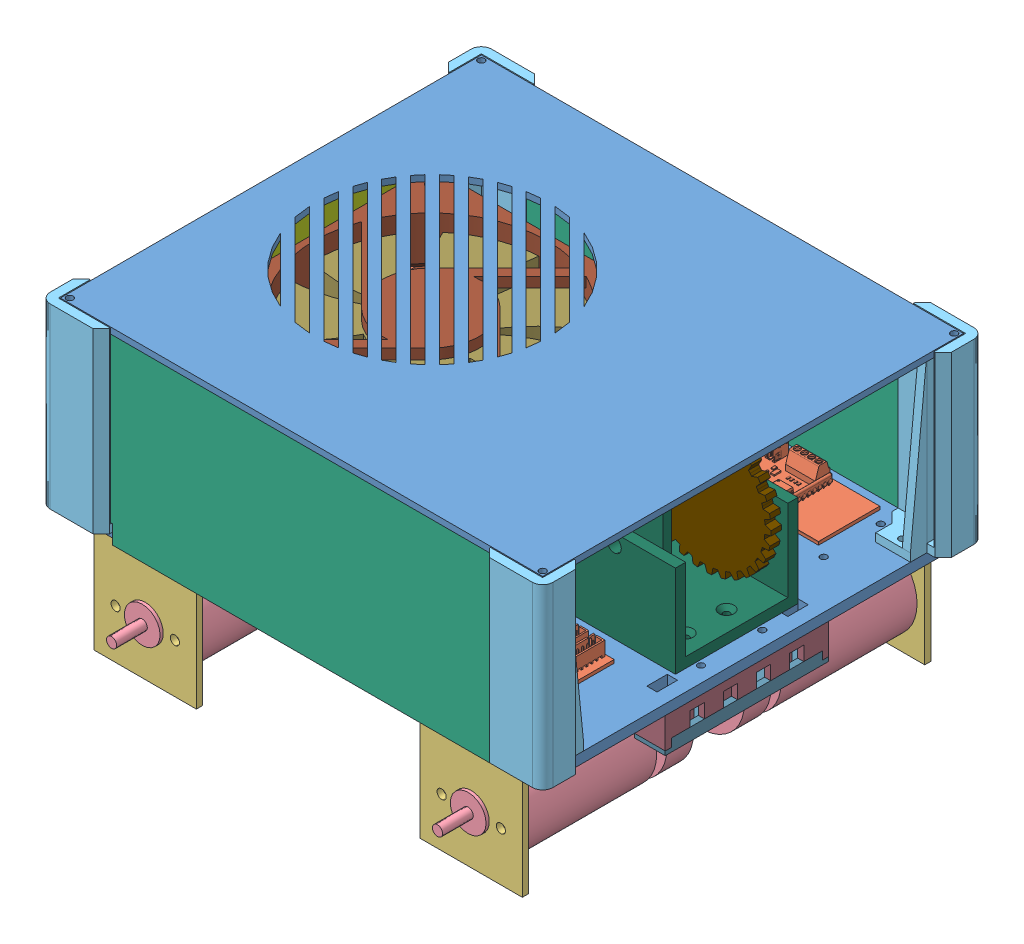
SolidWorks assembly SUM, configuration Standard. Lengths in mm.
Overall size (246 144 233).
34 component instances, 20 part files, 62 mates.
Components (placement in the parent):
- Part2^SUM-1: Part2^SUM [Standard] at origin (virtual)
- base_plate-1: base_plate [Standard] at (-44.1606 132.4921 37.7071) size (230 5 200)
- PCB_Chassisv1.0.step-1: PCB_Chassisv1.0.step [Standard] at (-139.1606 153.7785 -50.9871) x (0 0 1) z (0 1 0) size (160.04 200 38.68)
- motorhalter-1: motorhalter [Standard] at (40.8983 106.4921 129.0129) x (1 0 0) z (0 0 -1) size (50 52 55)
- motorhalter-2: motorhalter [Standard] at (-118.6423 106.4921 129.0129) x (1 0 0) z (0 0 -1) size (50 52 55)
- motorhalter-5: motorhalter [Standard] at (-119.1606 106.4921 -70.9871) x (-1 0 0) z (0 0 1) size (50 52 55)
- motorhalter-6: motorhalter [Standard] at (40.8394 106.4921 -70.9871) x (-1 0 0) z (0 0 1) size (50 52 55)
- motor-1: motor [Standard] at (-118.6423 104.4921 59.5129) size (42.5 42.5 104)
- motor-2: motor [Standard] at (40.8983 104.4921 59.5129) size (42.5 42.5 104)
- motor-3: motor [Standard] at (-119.1606 104.4921 -1.4871) x (1 0 0) z (0 0 -1) size (42.5 42.5 104)
- motor-4: motor [Standard] at (40.8394 104.4921 -1.4871) x (-1 0 0) z (0 0 -1) size (42.5 42.5 104)
- base-ecke-halter-2: base-ecke-halter [teil rechts] at (-147.1606 137.4921 -68.9871) x (0 0 -1) z (1 0 0) size (28 87 30)
- base-ecke-halter-3: base-ecke-halter [teil rechts] at (68.8394 137.4921 127.0129) x (0 0 1) z (-1 0 0) size (28 87 30)
- base-ecke-halter-6: base-ecke-halter [teil links] at (-147.1606 137.4921 127.0129) x (0 0 -1) z (1 0 0) size (28 87 30)
- base-ecke-halter-7: base-ecke-halter [teil links] at (68.8394 137.4921 -68.9871) x (0 0 1) z (-1 0 0) size (28 87 30)
- wall_L_R-1: wall_L_R [Standard] at (-39.1606 176.9921 129.0129) x (1 0 0) z (0 -1 0) size (227 3 89)
- wall_L_R-2: wall_L_R [Standard] at (-39.1606 176.9921 -73.9871) x (1 0 0) z (0 -1 0) size (227 3 89)
- wall_B-1: wall_B [Standard] at (-157.1606 176.9921 29.0129) x (0 0 -1) z (1 0 0) size (197 89 3)
- Funk.step-1: Funk.step [Standard] at (-80.8303 237.3371 119.9389) x (1 0 0) z (0 0 -1) size (61.6 64.9 16.02)
- LORA_mount-1: LORA_mount [Standard] at (-24.6323 144.9921 125.3504) x (-1 0 0) z (0 0 -1) size (70 75 15)
- Vent_mount-1: Vent_mount [Standard] at (-64.1606 178.4895 29.0129) x (0 0 1) z (-1 0 0) size (160 4 150)
- Vent.stp-1: Vent.stp [Standard] at (-139.9204 182.4895 90.0129) size (122.01 25.4 122.01)
  - FRAME.stp-1: FRAME.stp [Standard] at (61 0 -61) size (122.01 25.4 122.01)
  - 410005100005.stp-1: 410005100005.stp [Standard] at (61 2.0938 -61) x (1 0 0) z (0 -1 0) size (111.8 111.72 16)
- Scheinwerfer_Gehäuse-1: Scheinwerfer_Gehäuse [Standard] at (68.3394 132.4921 29.0129) x (0 0 1) z (1 0 0) size (80 15 15)
- Scheinwerfer_deckel-1: Scheinwerfer_deckel [Standard] at (68.3394 115.4921 29.0129) x (0 0 -1) z (1 0 0) size (80 6 15)
- Scheinwerfer_Gehäuse-2: Scheinwerfer_Gehäuse [Standard] at (-146.5449 132.4921 29.0134) x (0.007714 0 -0.99997) z (-0.99997 0 -0.007714) size (80 15 15)
- Scheinwerfer_deckel-2: Scheinwerfer_deckel [Standard] at (-146.5449 115.4921 29.0134) x (-0.007714 0 0.99997) z (-0.99997 0 -0.007714) size (80 6 15)
- seilwinde-1: seilwinde [Standard] at (70.9432 149.6596 27.3308) size (106.6 93.21 60)
  - seilwinde_case-1: seilwinde_case [Standard] at (-50.1038 -12.1675 -3.3179) size (90 45 60)
  - 858 Stepper Motor 5VDC.step-1: 858 Stepper Motor 5VDC.step [Standard] at (-72.6038 19.8325 -12.3221) x (-1 0 0) z (0 0 -1) size (42 34.5 29)
  - seilwinde_small_gear-1: seilwinde_small_gear [Standard] at (-72.5744 27.8557 -21.3221) x (1 0 0) z (0 -1 0) size (20.09 5 19.59)
  - seilwinde_big_gear-1: seilwinde_big_gear [Standard] at (-35.1038 27.8325 -17.1569) x (0.729284 -0.684211 0) z (0.684211 0.729284 0) size (65.88 15 66)
- roof1-1: roof1 [Standard] at (-39.1606 221.4921 29.0129) x (0 0 -1) z (1 0 0) size (206 3 236)
Mates (geometry in assembly coordinates):
- Slot1: slot anti-aligned: plane of motorhalter-1 through (49.6483 132.4921 115.7629) normal (0 0 1); cylinder of base_plate-1 through (52.3394 132.4921 118.0129) axis (0 1 0) radius 1.65; cylinder of motorhalter-1 through (55.1483 132.4921 118.0129) axis (0 -1 0) radius 2.25
- Slot2: slot anti-aligned: plane of motorhalter-1 through (26.6483 132.4921 115.7629) normal (0 0 1); cylinder of base_plate-1 through (29.3394 132.4921 118.0129) axis (0 1 0) radius 1.65; cylinder of motorhalter-1 through (32.1483 132.4921 118.0129) axis (0 -1 0) radius 2.25
- Coincident2: coincident anti-aligned: plane of base_plate-1 through (-44.1606 132.4921 37.7071) normal (0 -1 0); plane of motorhalter-1 through (15.8983 132.4921 126.0129) normal (0 1 0)
- Slot3: slot anti-aligned: plane of motorhalter-2 through (-132.8923 132.4921 115.7629) normal (0 0 1); cylinder of base_plate-1 through (-130.6606 132.4921 118.0129) axis (0 1 0) radius 1.65; cylinder of motorhalter-2 through (-127.3923 132.4921 118.0129) axis (0 -1 0) radius 2.25
- Slot4: slot anti-aligned: plane of motorhalter-2 through (-109.8923 132.4921 115.7629) normal (0 0 1); cylinder of base_plate-1 through (-107.6606 132.4921 118.0129) axis (0 1 0) radius 1.65; cylinder of motorhalter-2 through (-104.3923 132.4921 118.0129) axis (0 -1 0) radius 2.25
- Coincident3: coincident anti-aligned: plane of base_plate-1 through (-44.1606 132.4921 37.7071) normal (0 -1 0); plane of motorhalter-2 through (-143.6423 132.4921 126.0129) normal (0 1 0)
- Slot5: slot anti-aligned: plane of motorhalter-5 through (-127.9106 132.4921 -57.7371) normal (0 0 -1); cylinder of base_plate-1 through (-130.6606 132.4921 -59.9871) axis (0 1 0) radius 1.65; cylinder of motorhalter-5 through (-133.4106 132.4921 -59.9871) axis (0 -1 0) radius 2.25
- Slot6: slot anti-aligned: plane of motorhalter-5 through (-104.9106 132.4921 -57.7371) normal (0 0 -1); cylinder of base_plate-1 through (-107.6606 132.4921 -59.9871) axis (0 1 0) radius 1.65; cylinder of motorhalter-5 through (-110.4106 132.4921 -59.9871) axis (0 -1 0) radius 2.25
- Slot7: slot anti-aligned: plane of motorhalter-6 through (32.0894 132.4921 -57.7371) normal (0 0 -1); cylinder of base_plate-1 through (29.3394 132.4921 -59.9871) axis (0 1 0) radius 1.65; cylinder of motorhalter-6 through (26.5894 132.4921 -59.9871) axis (0 -1 0) radius 2.25
- Slot8: slot anti-aligned: plane of motorhalter-6 through (55.0894 132.4921 -57.7371) normal (0 0 -1); cylinder of base_plate-1 through (52.3394 132.4921 -59.9871) axis (0 1 0) radius 1.65; cylinder of motorhalter-6 through (49.5894 132.4921 -59.9871) axis (0 -1 0) radius 2.25
- Coincident4: coincident anti-aligned: plane of base_plate-1 through (-44.1606 132.4921 37.7071) normal (0 -1 0); plane of motorhalter-5 through (-94.1606 132.4921 -67.9871) normal (0 1 0)
- Coincident5: coincident anti-aligned: plane of base_plate-1 through (-44.1606 132.4921 37.7071) normal (0 -1 0); plane of motorhalter-6 through (65.8394 132.4921 -67.9871) normal (0 1 0)
- Concentric2: concentric anti-aligned: cylinder of motorhalter-2 through (-118.6423 104.4921 126.0129) axis (0 0 1) radius 8.8; cylinder of motor-1 through (-118.6423 104.4921 130.5129) axis (0 0 -1) radius 8.75
- Coincident7: coincident anti-aligned: plane of motorhalter-2 through (-118.6423 106.4921 126.0129) normal (0 0 -1); plane of motor-1 through (-118.6423 104.4921 126.0129) normal (0 0 1)
- Concentric3: concentric aligned: circle of motorhalter-1; cylinder of motor-2 through (40.8983 104.4921 130.5129) axis (0 0 -1) radius 8.75
- Concentric4: concentric anti-aligned: cylinder of motorhalter-5 through (-119.1606 104.4921 -67.9871) axis (0 0 -1) radius 8.8; cylinder of motor-3 through (-119.1606 104.4921 -72.4871) axis (0 0 1) radius 8.75
- Coincident8: coincident anti-aligned: plane of motorhalter-5 through (-119.1606 106.4921 -67.9871) normal (0 0 1); plane of motor-3 through (-119.1606 104.4921 -67.9871) normal (0 0 -1)
- Concentric5: concentric anti-aligned: circle of motorhalter-5; circle of motor-3
- Concentric6: concentric anti-aligned: cylinder of motorhalter-6 through (40.8394 104.4921 -67.9871) axis (0 0 -1) radius 8.8; cylinder of motor-4 through (40.8394 104.4921 -67.9871) axis (0 0 1) radius 21.25
- Coincident9: coincident anti-aligned: plane of motorhalter-6 through (40.8394 106.4921 -67.9871) normal (0 0 1); plane of motor-4 through (40.8394 104.4921 -67.9871) normal (0 0 -1)
- Concentric7: concentric anti-aligned: circle of motorhalter-6; circle of motor-4
- Deckungsgleich3: coincident aligned: circle of base_plate-1; circle of base-ecke-halter-2
- Deckungsgleich5: coincident aligned: circle of base_plate-1; circle of base-ecke-halter-3
- Coincident14: concentric anti-aligned: circle of base_plate-1; circle of base-ecke-halter-6
- Coincident15: coincident anti-aligned: circle of base_plate-1; cylinder of base-ecke-halter-6 through (-146.1606 141.4921 113.0129) axis (0 -1 0) radius 1.65
- Coincident16: coincident aligned: circle of base_plate-1; circle of base-ecke-halter-7
- Coincident17: coincident anti-aligned: circle of base_plate-1; circle of base-ecke-halter-7
- Coincident20: coincident aligned: line of base_plate-1 through (-154.1606 132.4921 129.0129) axis (1 0 0); line of wall_L_R-1 through (-131.6606 132.4921 129.0129) axis (1 0 0)
- Coincident21: coincident anti-aligned: plane of base-ecke-halter-7 through (68.8394 224.4921 -70.9871) normal (0 0 -1); plane of wall_L_R-2 through (-39.1606 176.9921 -70.9871) normal (0 0 1)
- Coincident23: coincident aligned: line of base_plate-1 through (-154.1606 132.4921 -70.9871) axis (1 0 0); line of wall_L_R-2 through (-131.6606 132.4921 -70.9871) axis (1 0 0)
- Deckungsgleich7: coincident anti-aligned: plane of base-ecke-halter-2 through (-154.1606 224.4921 -68.9871) normal (-1 0 0); plane of wall_B-1 through (-154.1606 176.9921 29.0129) normal (1 0 0)
- Deckungsgleich8: coincident aligned: line of base_plate-1 through (-154.1606 132.4921 129.0129) axis (0 0 -1); line of wall_B-1 through (-154.1606 132.4921 116.5129) axis (0 0 -1)
- Deckungsgleich9: coincident anti-aligned: plane of base-ecke-halter-6 through (-147.1606 224.4921 127.5129) normal (0 0 -1); plane of wall_B-1 through (-154.1606 176.9921 127.5129) normal (0 0 1)
- Deckungsgleich11: coincident anti-aligned: plane of base-ecke-halter-6 through (-152.6606 224.4921 127.0129) normal (1 0 0); plane of wall_L_R-1 through (-152.6606 176.9921 132.0129) normal (-1 0 0)
- Deckungsgleich12: coincident anti-aligned: plane of base-ecke-halter-2 through (-152.6606 224.4921 -68.9871) normal (1 0 0); plane of wall_L_R-2 through (-152.6606 176.9921 -70.9871) normal (-1 0 0)
- Deckungsgleich15: coincident aligned: circle of base_plate-1; circle of LORA_mount-1
- Deckungsgleich16: coincident aligned: circle of base_plate-1; circle of LORA_mount-1
- Konzentrisch5: concentric aligned: circle of Funk.step-1; circle of LORA_mount-1
- Parallel10: parallel anti-aligned: line of Funk.step-1 through (-55.4303 210.5401 120.3504) axis (1 0 0); line of LORA_mount-1 through (-0.6323 152.4921 120.3504) axis (-1 0 0)
- Deckungsgleich18: coincident anti-aligned: plane of Funk.step-1 through (-55.4303 210.5401 120.3504) normal (0 0 1); plane of LORA_mount-1 through (-24.6323 144.9921 120.3504) normal (0 0 -1)
- Konzentrisch8: concentric aligned: circle of base_plate-1; circle of PCB_Chassisv1.0.step-1
- Konzentrisch9: concentric aligned: circle of base_plate-1; circle of PCB_Chassisv1.0.step-1
- Coincident24: coincident anti-aligned: plane of motorhalter-1 through (40.8983 106.4921 126.0129) normal (0 0 -1); plane of motor-2 through (40.8983 104.4921 126.0129) normal (0 0 1)
- Concentric8: concentric aligned: circle of base_plate-1; circle of Vent_mount-1
- Concentric9: concentric aligned: circle of base_plate-1; circle of Vent_mount-1
- Coincident27: coincident anti-aligned: circle of Vent_mount-1; circle of Vent.stp-1/FRAME.stp-1
- Coincident28: coincident anti-aligned: circle of Vent_mount-1; circle of Vent.stp-1/FRAME.stp-1
- Deckungsgleich19: coincident anti-aligned: circle of base_plate-1; circle of Scheinwerfer_Gehäuse-1
- Deckungsgleich20: coincident anti-aligned: circle of base_plate-1; circle of Scheinwerfer_Gehäuse-1
- Konzentrisch10: concentric anti-aligned: circle of Scheinwerfer_Gehäuse-1; circle of Scheinwerfer_deckel-1
- Deckungsgleich23: coincident anti-aligned: plane of Scheinwerfer_Gehäuse-1 through (70.8394 121.4921 29.0129) normal (0 -1 0); plane of Scheinwerfer_deckel-1 through (68.3394 121.4921 29.0129) normal (0 1 0)
- Deckungsgleich24: coincident anti-aligned: line of Scheinwerfer_Gehäuse-1 through (60.8394 117.4921 -10.9871) axis (1 0 0); line of Scheinwerfer_deckel-1 through (75.8394 117.4921 -10.9871) axis (-1 0 0)
- Konzentrisch11: concentric anti-aligned: circle of Scheinwerfer_Gehäuse-2; circle of Scheinwerfer_deckel-2
- Deckungsgleich25: coincident anti-aligned: plane of Scheinwerfer_Gehäuse-2 through (-149.0448 121.4921 28.9941) normal (0 -1 0); plane of Scheinwerfer_deckel-2 through (-146.5449 121.4921 29.0134) normal (0 1 0)
- Deckungsgleich26: coincident anti-aligned: line of Scheinwerfer_Gehäuse-2 through (-139.3537 117.4921 69.07) axis (-0.99997 0 -0.007714); line of Scheinwerfer_deckel-2 through (-154.3533 117.4921 68.9543) axis (0.99997 0 0.007714)
- Deckungsgleich29: coincident anti-aligned: circle of base_plate-1; circle of Scheinwerfer_Gehäuse-2
- Konzentrisch12: concentric aligned: circle of base_plate-1; circle of base-ecke-halter-2
- Deckungsgleich30: coincident aligned: circle of base_plate-1; circle of seilwinde-1/seilwinde_case-1
- Parallel11: parallel anti-aligned: line of wall_B-1 through (-157.1606 221.4921 127.5129) axis (0 0 -1); line of roof1-1 through (-157.1606 221.4921 -73.9871) axis (0 0 1)
- Parallel12: parallel anti-aligned: line of wall_L_R-2 through (-152.6606 221.4921 -73.9871) axis (1 0 0); line of roof1-1 through (78.8394 221.4921 -73.9871) axis (-1 0 0)
- Konzentrisch16: concentric aligned: circle of base-ecke-halter-2; circle of roof1-1
- Deckungsgleich33: coincident anti-aligned: plane of base-ecke-halter-2 through (-147.1606 221.4921 -68.9871) normal (0 1 0); plane of roof1-1 through (-39.1606 221.4921 29.0129) normal (0 -1 0)
